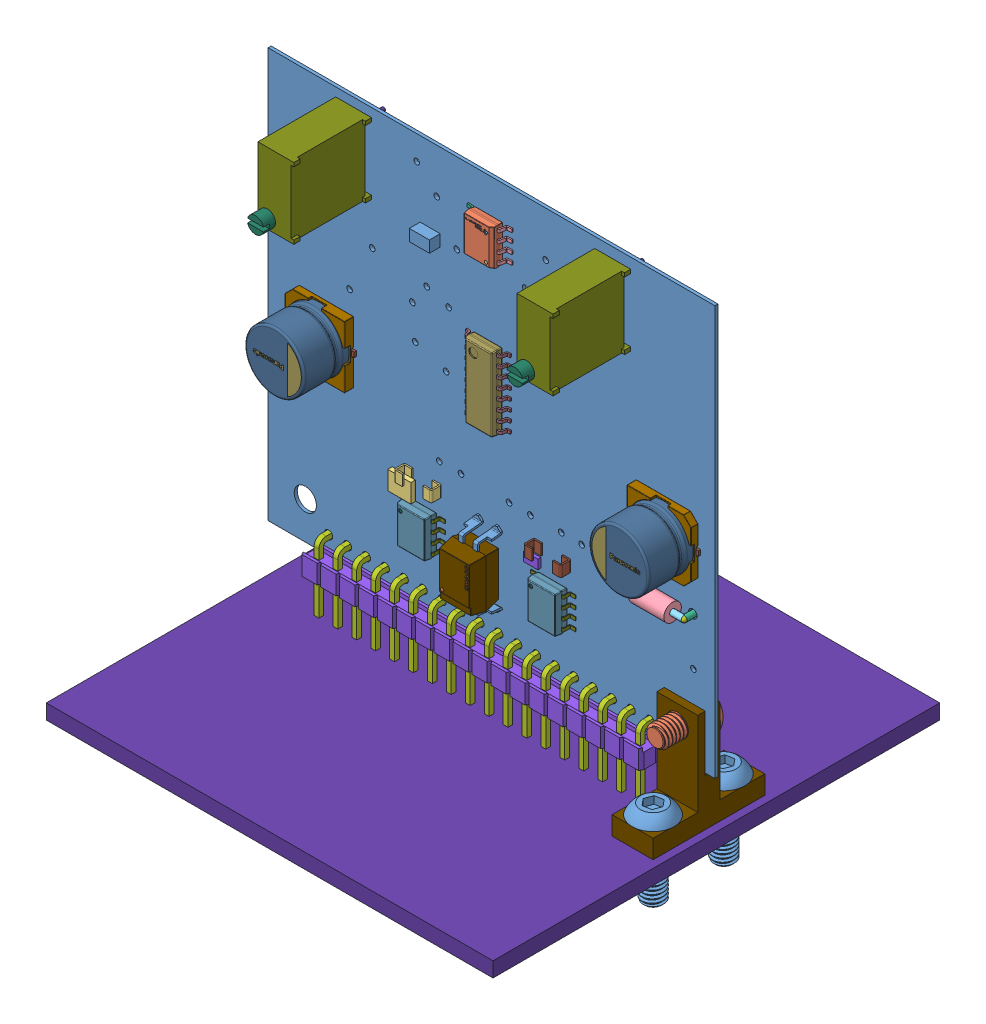
SolidWorks assembly Макет PWM, configuration Default. Lengths in mm.
Overall size (60 68.93 60).
439 component instances, 56 part files, 6 mates.
Components (placement in the parent):
- PWM_controller-1: PWM_controller [Default] at (-319.0135 -82.8288 51.7656) size (60 62.62 16.05)
  - PWM_controller.step-1: PWM_controller.step [Default] at origin size (60 62.62 16.05)
    - Board.step-1: Board.step [Default] at origin size (60 55 0.41)
      - Open CASCADE STEP translator 6.8 2.1.1.step-1: Open CASCADE STEP translator 6.8 2.1.1.step [Default] at (0 0 -0.4115) size (60 55 0.41)
    - R32.step-1: R32.step [Default] at origin size (3.2 2.5 0.7)
      - Res_Stackpole_Electronics_RMCF1210JT5K10_eec.step-1: Res_Stackpole_Electronics_RMCF1210JT5K10_eec.step [Default] at (249.8598 58.1914 -0.4115) x (-1 0 0) z (0 0 -1) size (3.2 2.5 0.7)
        - terminals.step-1: terminals.step [Default] at origin size (3.2 2.5 0.7)
        - body.step-1: body.step [Default] at origin size (3.1 2.5 0.6)
        - top.step-1: top.step [Default] at (-0.71 0 0.65) size (2.2 2.5 0.05)
        - logo.step-1: logo.step [Default] at (0 0 0.7) size (1.25 0.57 0)
    - C2.step-1: C2.step [Default] at origin size (2.7 3.4 1)
      - 6948496496.step-1: 6948496496.step [Default] at (219.9386 58.9514 -1.4115) size (2.7 0.5 1)
        - Extruded.step-1: Extruded.step [Default] at origin size (2.7 0.5 1)
      - 6948496496.step-2: 6948496496.step [Default] at (219.9386 61.8514 -1.4115) size (2.7 0.5 1)
        - Extruded.step-1: Extruded.step [Default] at origin size (2.7 0.5 1)
      - 6948486416.step-1: 6948486416.step [Default] at (219.9386 60.4014 -1.4115) size (2.7 2.4 1)
        - Extruded-0.step-1: Extruded-0.step [Default] at origin size (2.7 2.4 1)
    - C1.step-1: C1.step [Default] at origin size (2.7 3.4 1)
      - 6948496496.step-1: 6948496496.step [Default] at (237.0328 57.9862 -1.4115) size (2.7 0.5 1)
        - Extruded.step-1: Extruded.step [Default] at origin size (2.7 0.5 1)
      - 6948496496.step-2: 6948496496.step [Default] at (237.0328 60.8862 -1.4115) size (2.7 0.5 1)
        - Extruded.step-1: Extruded.step [Default] at origin size (2.7 0.5 1)
      - 6948486416.step-1: 6948486416.step [Default] at (237.0328 59.4362 -1.4115) size (2.7 2.4 1)
        - Extruded-0.step-1: Extruded-0.step [Default] at origin size (2.7 2.4 1)
    - R31.step-1: R31.step [Default] at origin size (1.25 2 0.5)
      - Res_Vishay_CRCW0805100KFKEA_eec.step-1: Res_Vishay_CRCW0805100KFKEA_eec.step [Default] at (205.232 89.4842 -0.4115) x (0 1 0) z (0 0 -1) size (2 1.25 0.5)
        - body-1.step-1: body-1.step [Default] at (0 0 0.45) x (1 0 0) z (0 0 -1) size (1.9 1.25 0.4)
        - pad.step-1: pad.step [Default] at (-0.8133 -0.625 0.5) x (1 0 0) z (0 1 0) size (0.3 0.5 1.25)
        - pad.step-2: pad.step [Default] at (0.8133 0.625 0.5) x (-1 0 0) z (0 -1 0) size (0.3 0.5 1.25)
        - top-2.step-1: top-2.step [Default] at (0 0 0.05) x (1 0 0) z (0 0 -1) size (1.4 1.25 0.05)
        - top-2.step-2: top-2.step [Default] at (0 0 0.5) x (1 0 0) z (0 0 -1) size (1.4 1.25 0.05)
        - Vishay.step-1: Vishay.step [Default] at (0.032 -0.7832 0.5) size (0.44 0.37 0)
    - R4.step-1: R4.step [Default] at origin size (1.25 2 0.5)
      - Res_Vishay_CRCW0805100KFKEA_eec.step-1: Res_Vishay_CRCW0805100KFKEA_eec.step [Default] at (206.9846 87.503 -0.4115) x (0 -1 0) z (0 0 -1) size (2 1.25 0.5)
        - body-1.step-1: body-1.step [Default] at (0 0 0.45) x (1 0 0) z (0 0 -1) size (1.9 1.25 0.4)
        - pad.step-1: pad.step [Default] at (-0.8133 -0.625 0.5) x (1 0 0) z (0 1 0) size (0.3 0.5 1.25)
        - pad.step-2: pad.step [Default] at (0.8133 0.625 0.5) x (-1 0 0) z (0 -1 0) size (0.3 0.5 1.25)
        - top-2.step-1: top-2.step [Default] at (0 0 0.05) x (1 0 0) z (0 0 -1) size (1.4 1.25 0.05)
        - top-2.step-2: top-2.step [Default] at (0 0 0.5) x (1 0 0) z (0 0 -1) size (1.4 1.25 0.05)
        - Vishay.step-1: Vishay.step [Default] at (0.032 -0.7832 0.5) size (0.44 0.37 0)
    - R3.step-1: R3.step [Default] at origin size (1.25 2 0.5)
      - Res_Vishay_CRCW0805100KFKEA_eec.step-1: Res_Vishay_CRCW0805100KFKEA_eec.step [Default] at (210.3628 76.8604 -0.4115) x (0 -1 0) z (0 0 -1) size (2 1.25 0.5)
        - body-1.step-1: body-1.step [Default] at (0 0 0.45) x (1 0 0) z (0 0 -1) size (1.9 1.25 0.4)
        - pad.step-1: pad.step [Default] at (-0.8133 -0.625 0.5) x (1 0 0) z (0 1 0) size (0.3 0.5 1.25)
        - pad.step-2: pad.step [Default] at (0.8133 0.625 0.5) x (-1 0 0) z (0 -1 0) size (0.3 0.5 1.25)
        - top-2.step-1: top-2.step [Default] at (0 0 0.05) x (1 0 0) z (0 0 -1) size (1.4 1.25 0.05)
        - top-2.step-2: top-2.step [Default] at (0 0 0.5) x (1 0 0) z (0 0 -1) size (1.4 1.25 0.05)
        - Vishay.step-1: Vishay.step [Default] at (0.032 -0.7832 0.5) size (0.44 0.37 0)
    - R2.step-1: R2.step [Default] at origin size (1.25 2 0.5)
      - Res_Vishay_CRCW0805100KFKEA_eec.step-1: Res_Vishay_CRCW0805100KFKEA_eec.step [Default] at (223.7232 76.7588 -0.4115) x (0 -1 0) z (0 0 -1) size (2 1.25 0.5)
        - body-1.step-1: body-1.step [Default] at (0 0 0.45) x (1 0 0) z (0 0 -1) size (1.9 1.25 0.4)
        - pad.step-1: pad.step [Default] at (-0.8133 -0.625 0.5) x (1 0 0) z (0 1 0) size (0.3 0.5 1.25)
        - pad.step-2: pad.step [Default] at (0.8133 0.625 0.5) x (-1 0 0) z (0 -1 0) size (0.3 0.5 1.25)
        - top-2.step-1: top-2.step [Default] at (0 0 0.05) x (1 0 0) z (0 0 -1) size (1.4 1.25 0.05)
        - top-2.step-2: top-2.step [Default] at (0 0 0.5) x (1 0 0) z (0 0 -1) size (1.4 1.25 0.05)
        - Vishay.step-1: Vishay.step [Default] at (0.032 -0.7832 0.5) size (0.44 0.37 0)
    - R1.step-1: R1.step [Default] at origin size (1.25 2 0.5)
      - Res_Vishay_CRCW0805100KFKEA_eec.step-1: Res_Vishay_CRCW0805100KFKEA_eec.step [Default] at (225.7044 76.7842 -0.4115) x (0 1 0) z (0 0 -1) size (2 1.25 0.5)
        - body-1.step-1: body-1.step [Default] at (0 0 0.45) x (1 0 0) z (0 0 -1) size (1.9 1.25 0.4)
        - pad.step-1: pad.step [Default] at (-0.8133 -0.625 0.5) x (1 0 0) z (0 1 0) size (0.3 0.5 1.25)
        - pad.step-2: pad.step [Default] at (0.8133 0.625 0.5) x (-1 0 0) z (0 -1 0) size (0.3 0.5 1.25)
        - top-2.step-1: top-2.step [Default] at (0 0 0.05) x (1 0 0) z (0 0 -1) size (1.4 1.25 0.05)
        - top-2.step-2: top-2.step [Default] at (0 0 0.5) x (1 0 0) z (0 0 -1) size (1.4 1.25 0.05)
        - Vishay.step-1: Vishay.step [Default] at (0.032 -0.7832 0.5) size (0.44 0.37 0)
    - R30.step-1: R30.step [Default] at origin size (1.25 2 0.5)
      - Res_Vishay_CRCW0805100KFKEA_eec.step-1: Res_Vishay_CRCW0805100KFKEA_eec.step [Default] at (220.9546 82.6008 -0.4115) x (0 -1 0) z (0 0 -1) size (2 1.25 0.5)
        - body-1.step-1: body-1.step [Default] at (0 0 0.45) x (1 0 0) z (0 0 -1) size (1.9 1.25 0.4)
        - pad.step-1: pad.step [Default] at (-0.8133 -0.625 0.5) x (1 0 0) z (0 1 0) size (0.3 0.5 1.25)
        - pad.step-2: pad.step [Default] at (0.8133 0.625 0.5) x (-1 0 0) z (0 -1 0) size (0.3 0.5 1.25)
        - top-2.step-1: top-2.step [Default] at (0 0 0.05) x (1 0 0) z (0 0 -1) size (1.4 1.25 0.05)
        - top-2.step-2: top-2.step [Default] at (0 0 0.5) x (1 0 0) z (0 0 -1) size (1.4 1.25 0.05)
        - Vishay.step-1: Vishay.step [Default] at (0.032 -0.7832 0.5) size (0.44 0.37 0)
    - R29.step-1: R29.step [Default] at origin size (1.25 2 0.5)
      - Res_Vishay_CRCW0805100KFKEA_eec.step-1: Res_Vishay_CRCW0805100KFKEA_eec.step [Default] at (211.2772 90.4084 -0.4115) x (0 -1 0) z (0 0 -1) size (2 1.25 0.5)
        - body-1.step-1: body-1.step [Default] at (0 0 0.45) x (1 0 0) z (0 0 -1) size (1.9 1.25 0.4)
        - pad.step-1: pad.step [Default] at (-0.8133 -0.625 0.5) x (1 0 0) z (0 1 0) size (0.3 0.5 1.25)
        - pad.step-2: pad.step [Default] at (0.8133 0.625 0.5) x (-1 0 0) z (0 -1 0) size (0.3 0.5 1.25)
        - top-2.step-1: top-2.step [Default] at (0 0 0.05) x (1 0 0) z (0 0 -1) size (1.4 1.25 0.05)
        - top-2.step-2: top-2.step [Default] at (0 0 0.5) x (1 0 0) z (0 0 -1) size (1.4 1.25 0.05)
        - Vishay.step-1: Vishay.step [Default] at (0.032 -0.7832 0.5) size (0.44 0.37 0)
    - R28.step-1: R28.step [Default] at origin size (2 1.25 0.5)
      - Res_Vishay_CRCW0805100KFKEA_eec.step-1: Res_Vishay_CRCW0805100KFKEA_eec.step [Default] at (224.0026 85.6742 -0.4115) x (-1 0 0) z (0 0 -1) size (2 1.25 0.5)
        - body-1.step-1: body-1.step [Default] at (0 0 0.45) x (1 0 0) z (0 0 -1) size (1.9 1.25 0.4)
        - pad.step-1: pad.step [Default] at (-0.8133 -0.625 0.5) x (1 0 0) z (0 1 0) size (0.3 0.5 1.25)
        - pad.step-2: pad.step [Default] at (0.8133 0.625 0.5) x (-1 0 0) z (0 -1 0) size (0.3 0.5 1.25)
        - top-2.step-1: top-2.step [Default] at (0 0 0.05) x (1 0 0) z (0 0 -1) size (1.4 1.25 0.05)
        - top-2.step-2: top-2.step [Default] at (0 0 0.5) x (1 0 0) z (0 0 -1) size (1.4 1.25 0.05)
        - Vishay.step-1: Vishay.step [Default] at (0.032 -0.7832 0.5) size (0.44 0.37 0)
    - R27.step-1: R27.step [Default] at origin size (1.25 2 0.5)
      - Res_Vishay_CRCW0805100KFKEA_eec.step-1: Res_Vishay_CRCW0805100KFKEA_eec.step [Default] at (213.7156 87.5792 -0.4115) x (0 -1 0) z (0 0 -1) size (2 1.25 0.5)
        - body-1.step-1: body-1.step [Default] at (0 0 0.45) x (1 0 0) z (0 0 -1) size (1.9 1.25 0.4)
        - pad.step-1: pad.step [Default] at (-0.8133 -0.625 0.5) x (1 0 0) z (0 1 0) size (0.3 0.5 1.25)
        - pad.step-2: pad.step [Default] at (0.8133 0.625 0.5) x (-1 0 0) z (0 -1 0) size (0.3 0.5 1.25)
        - top-2.step-1: top-2.step [Default] at (0 0 0.05) x (1 0 0) z (0 0 -1) size (1.4 1.25 0.05)
        - top-2.step-2: top-2.step [Default] at (0 0 0.5) x (1 0 0) z (0 0 -1) size (1.4 1.25 0.05)
        - Vishay.step-1: Vishay.step [Default] at (0.032 -0.7832 0.5) size (0.44 0.37 0)
    - C14.step-1: C14.step [Default] at origin size (1.25 2 0.88)
      - Cap_KEMET_C0805C472J3HAC_eec.step-1: Cap_KEMET_C0805C472J3HAC_eec.step [Default] at (211.2264 84.3788 -0.4115) x (0 1 0) z (0 0 -1) size (1 1.15 0.78)
      - Cap_KEMET_C0805C472J3HAC_eec-3.step-1: Cap_KEMET_C0805C472J3HAC_eec-3.step [Default] at (211.2264 84.3788 -0.4115) x (0 1 0) z (0 0 -1) size (2 1.25 0.88)
      - Cap_KEMET_C0805C472J3HAC_eec-4.step-1: Cap_KEMET_C0805C472J3HAC_eec-4.step [Default] at (211.2264 84.3788 -0.4115) x (0 1 0) z (0 0 -1) size (0.59 0.12 0)
    - C13.step-1: C13.step [Default] at origin size (1.25 2 0.88)
      - Cap_KEMET_C0805C472J3HAC_eec.step-1: Cap_KEMET_C0805C472J3HAC_eec.step [Default] at (213.6648 84.3788 -0.4115) x (0 -1 0) z (0 0 -1) size (1 1.15 0.78)
      - Cap_KEMET_C0805C472J3HAC_eec-3.step-1: Cap_KEMET_C0805C472J3HAC_eec-3.step [Default] at (213.6648 84.3788 -0.4115) x (0 -1 0) z (0 0 -1) size (2 1.25 0.88)
      - Cap_KEMET_C0805C472J3HAC_eec-4.step-1: Cap_KEMET_C0805C472J3HAC_eec-4.step [Default] at (213.6648 84.3788 -0.4115) x (0 -1 0) z (0 0 -1) size (0.59 0.12 0)
    - R21.step-1: R21.step [Default] at origin size (2 1.25 0.5)
      - Res_Vishay_CRCW0805100KFKEA_eec.step-1: Res_Vishay_CRCW0805100KFKEA_eec.step [Default] at (225.0694 92.8624 -0.4115) x (1 0 0) z (0 0 -1) size (2 1.25 0.5)
        - body-1.step-1: body-1.step [Default] at (0 0 0.45) x (1 0 0) z (0 0 -1) size (1.9 1.25 0.4)
        - pad.step-1: pad.step [Default] at (-0.8133 -0.625 0.5) x (1 0 0) z (0 1 0) size (0.3 0.5 1.25)
        - pad.step-2: pad.step [Default] at (0.8133 0.625 0.5) x (-1 0 0) z (0 -1 0) size (0.3 0.5 1.25)
        - top-2.step-1: top-2.step [Default] at (0 0 0.05) x (1 0 0) z (0 0 -1) size (1.4 1.25 0.05)
        - top-2.step-2: top-2.step [Default] at (0 0 0.5) x (1 0 0) z (0 0 -1) size (1.4 1.25 0.05)
        - Vishay.step-1: Vishay.step [Default] at (0.032 -0.7832 0.5) size (0.44 0.37 0)
    - R20.step-1: R20.step [Default] at origin size (1.25 2 0.5)
      - Res_Vishay_CRCW0805100KFKEA_eec.step-1: Res_Vishay_CRCW0805100KFKEA_eec.step [Default] at (216.7382 97.3074 -0.4115) x (0 -1 0) z (0 0 -1) size (2 1.25 0.5)
        - body-1.step-1: body-1.step [Default] at (0 0 0.45) x (1 0 0) z (0 0 -1) size (1.9 1.25 0.4)
        - pad.step-1: pad.step [Default] at (-0.8133 -0.625 0.5) x (1 0 0) z (0 1 0) size (0.3 0.5 1.25)
        - pad.step-2: pad.step [Default] at (0.8133 0.625 0.5) x (-1 0 0) z (0 -1 0) size (0.3 0.5 1.25)
        - top-2.step-1: top-2.step [Default] at (0 0 0.05) x (1 0 0) z (0 0 -1) size (1.4 1.25 0.05)
        - top-2.step-2: top-2.step [Default] at (0 0 0.5) x (1 0 0) z (0 0 -1) size (1.4 1.25 0.05)
        - Vishay.step-1: Vishay.step [Default] at (0.032 -0.7832 0.5) size (0.44 0.37 0)
    - R19.step-1: R19.step [Default] at origin size (4.83 9.53 16.05)
      - Res_Bourns_3296W-1-504LF_eec.step-1: Res_Bourns_3296W-1-504LF_eec.step [Default] at (210.3653 92.9274 10.0159) x (0 0 -1) z (-1 0 0) size (1.59 2.18 2.18)
      - Res_Bourns_3296W-1-504LF_eec-5.step-1: Res_Bourns_3296W-1-504LF_eec-5.step [Default] at (210.3653 92.9274 10.0159) x (0 0 -1) z (-1 0 0) size (10.46 9.53 4.83)
      - Res_Bourns_3296W-1-504LF_eec-6.step-1: Res_Bourns_3296W-1-504LF_eec-6.step [Default] at (210.3653 92.9274 10.0159) x (0 0 -1) z (-1 0 0) size (4.53 5.59 0.51)
      - Res_Bourns_3296W-1-504LF_eec-7.step-1: Res_Bourns_3296W-1-504LF_eec-7.step [Default] at (210.3653 92.9274 10.0159) x (0 0 -1) z (-1 0 0) size (0.78 6.02 0.01)
    - R18.step-1: R18.step [Default] at origin size (1.25 2 0.5)
      - Res_Vishay_CRCW0805100KFKEA_eec.step-1: Res_Vishay_CRCW0805100KFKEA_eec.step [Default] at (214.884 97.3328 -0.4115) x (0 -1 0) z (0 0 -1) size (2 1.25 0.5)
        - body-1.step-1: body-1.step [Default] at (0 0 0.45) x (1 0 0) z (0 0 -1) size (1.9 1.25 0.4)
        - pad.step-1: pad.step [Default] at (-0.8133 -0.625 0.5) x (1 0 0) z (0 1 0) size (0.3 0.5 1.25)
        - pad.step-2: pad.step [Default] at (0.8133 0.625 0.5) x (-1 0 0) z (0 -1 0) size (0.3 0.5 1.25)
        - top-2.step-1: top-2.step [Default] at (0 0 0.05) x (1 0 0) z (0 0 -1) size (1.4 1.25 0.05)
        - top-2.step-2: top-2.step [Default] at (0 0 0.5) x (1 0 0) z (0 0 -1) size (1.4 1.25 0.05)
        - Vishay.step-1: Vishay.step [Default] at (0.032 -0.7832 0.5) size (0.44 0.37 0)
    - R17.step-1: R17.step [Default] at origin size (2 1.25 0.5)
      - Res_Vishay_CRCW0805100KFKEA_eec.step-1: Res_Vishay_CRCW0805100KFKEA_eec.step [Default] at (222.631 97.6376 -0.4115) x (-1 0 0) z (0 0 -1) size (2 1.25 0.5)
        - body-1.step-1: body-1.step [Default] at (0 0 0.45) x (1 0 0) z (0 0 -1) size (1.9 1.25 0.4)
        - pad.step-1: pad.step [Default] at (-0.8133 -0.625 0.5) x (1 0 0) z (0 1 0) size (0.3 0.5 1.25)
        - pad.step-2: pad.step [Default] at (0.8133 0.625 0.5) x (-1 0 0) z (0 -1 0) size (0.3 0.5 1.25)
        - top-2.step-1: top-2.step [Default] at (0 0 0.05) x (1 0 0) z (0 0 -1) size (1.4 1.25 0.05)
        - top-2.step-2: top-2.step [Default] at (0 0 0.5) x (1 0 0) z (0 0 -1) size (1.4 1.25 0.05)
        - Vishay.step-1: Vishay.step [Default] at (0.032 -0.7832 0.5) size (0.44 0.37 0)
    - D5.step-1: D5.step [Default] at origin size (2.7 1.55 1.45)
      - 6038362448.step-1: 6038362448.step [Default] at (235.0262 92.964 0) size (2.7 1.55 1.45)
        - Extruded-8.step-1: Extruded-8.step [Default] at origin size (2.7 1.55 1.45)
    - D4.step-1: D4.step [Default] at origin size (2.7 1.55 1.45)
      - 6038362448.step-1: 6038362448.step [Default] at (218.6178 92.7862 0) size (2.7 1.55 1.45)
        - Extruded-8.step-1: Extruded-8.step [Default] at origin size (2.7 1.55 1.45)
    - C12.step-1: C12.step [Default] at origin size (2 1.25 0.88)
      - Cap_KEMET_C0805C472J3HAC_eec.step-1: Cap_KEMET_C0805C472J3HAC_eec.step [Default] at (237.2614 97.9424 -0.4115) x (1 0 0) z (0 0 -1) size (1 1.15 0.78)
      - Cap_KEMET_C0805C472J3HAC_eec-3.step-1: Cap_KEMET_C0805C472J3HAC_eec-3.step [Default] at (237.2614 97.9424 -0.4115) x (1 0 0) z (0 0 -1) size (2 1.25 0.88)
      - Cap_KEMET_C0805C472J3HAC_eec-4.step-1: Cap_KEMET_C0805C472J3HAC_eec-4.step [Default] at (237.2614 97.9424 -0.4115) x (1 0 0) z (0 0 -1) size (0.59 0.12 0)
    - C11.step-1: C11.step [Default] at origin size (1.25 2 0.88)
      - Cap_KEMET_C0805C472J3HAC_eec.step-1: Cap_KEMET_C0805C472J3HAC_eec.step [Default] at (212.6996 97.3836 -0.4115) x (0 -1 0) z (0 0 -1) size (1 1.15 0.78)
      - Cap_KEMET_C0805C472J3HAC_eec-3.step-1: Cap_KEMET_C0805C472J3HAC_eec-3.step [Default] at (212.6996 97.3836 -0.4115) x (0 -1 0) z (0 0 -1) size (2 1.25 0.88)
      - Cap_KEMET_C0805C472J3HAC_eec-4.step-1: Cap_KEMET_C0805C472J3HAC_eec-4.step [Default] at (212.6996 97.3836 -0.4115) x (0 -1 0) z (0 0 -1) size (0.59 0.12 0)
    - R25.step-1: R25.step [Default] at origin size (2 1.25 0.5)
      - Res_Vishay_CRCW0805100KFKEA_eec.step-1: Res_Vishay_CRCW0805100KFKEA_eec.step [Default] at (231.2416 97.663 -0.4115) x (-1 0 0) z (0 0 -1) size (2 1.25 0.5)
        - body-1.step-1: body-1.step [Default] at (0 0 0.45) x (1 0 0) z (0 0 -1) size (1.9 1.25 0.4)
        - pad.step-1: pad.step [Default] at (-0.8133 -0.625 0.5) x (1 0 0) z (0 1 0) size (0.3 0.5 1.25)
        - pad.step-2: pad.step [Default] at (0.8133 0.625 0.5) x (-1 0 0) z (0 -1 0) size (0.3 0.5 1.25)
        - top-2.step-1: top-2.step [Default] at (0 0 0.05) x (1 0 0) z (0 0 -1) size (1.4 1.25 0.05)
        - top-2.step-2: top-2.step [Default] at (0 0 0.5) x (1 0 0) z (0 0 -1) size (1.4 1.25 0.05)
        - Vishay.step-1: Vishay.step [Default] at (0.032 -0.7832 0.5) size (0.44 0.37 0)
    - R23.step-1: R23.step [Default] at origin size (2 1.25 0.5)
      - Res_Vishay_CRCW0805100KFKEA_eec.step-1: Res_Vishay_CRCW0805100KFKEA_eec.step [Default] at (237.2614 100.1268 -0.4115) x (1 0 0) z (0 0 -1) size (2 1.25 0.5)
        - body-1.step-1: body-1.step [Default] at (0 0 0.45) x (1 0 0) z (0 0 -1) size (1.9 1.25 0.4)
        - pad.step-1: pad.step [Default] at (-0.8133 -0.625 0.5) x (1 0 0) z (0 1 0) size (0.3 0.5 1.25)
        - pad.step-2: pad.step [Default] at (0.8133 0.625 0.5) x (-1 0 0) z (0 -1 0) size (0.3 0.5 1.25)
        - top-2.step-1: top-2.step [Default] at (0 0 0.05) x (1 0 0) z (0 0 -1) size (1.4 1.25 0.05)
        - top-2.step-2: top-2.step [Default] at (0 0 0.5) x (1 0 0) z (0 0 -1) size (1.4 1.25 0.05)
        - Vishay.step-1: Vishay.step [Default] at (0.032 -0.7832 0.5) size (0.44 0.37 0)
    - R26.step-1: R26.step [Default] at origin size (2 1.25 0.5)
      - Res_Vishay_CRCW0805100KFKEA_eec.step-1: Res_Vishay_CRCW0805100KFKEA_eec.step [Default] at (228.6508 92.8624 -0.4115) x (-1 0 0) z (0 0 -1) size (2 1.25 0.5)
        - body-1.step-1: body-1.step [Default] at (0 0 0.45) x (1 0 0) z (0 0 -1) size (1.9 1.25 0.4)
        - pad.step-1: pad.step [Default] at (-0.8133 -0.625 0.5) x (1 0 0) z (0 1 0) size (0.3 0.5 1.25)
        - pad.step-2: pad.step [Default] at (0.8133 0.625 0.5) x (-1 0 0) z (0 -1 0) size (0.3 0.5 1.25)
        - top-2.step-1: top-2.step [Default] at (0 0 0.05) x (1 0 0) z (0 0 -1) size (1.4 1.25 0.05)
        - top-2.step-2: top-2.step [Default] at (0 0 0.5) x (1 0 0) z (0 0 -1) size (1.4 1.25 0.05)
        - Vishay.step-1: Vishay.step [Default] at (0.032 -0.7832 0.5) size (0.44 0.37 0)
    - R22.step-1: R22.step [Default] at origin size (2 1.25 0.5)
      - Res_Vishay_CRCW0805100KFKEA_eec.step-1: Res_Vishay_CRCW0805100KFKEA_eec.step [Default] at (234.2388 95.2754 -0.4115) x (1 0 0) z (0 0 -1) size (2 1.25 0.5)
        - body-1.step-1: body-1.step [Default] at (0 0 0.45) x (1 0 0) z (0 0 -1) size (1.9 1.25 0.4)
        - pad.step-1: pad.step [Default] at (-0.8133 -0.625 0.5) x (1 0 0) z (0 1 0) size (0.3 0.5 1.25)
        - pad.step-2: pad.step [Default] at (0.8133 0.625 0.5) x (-1 0 0) z (0 -1 0) size (0.3 0.5 1.25)
        - top-2.step-1: top-2.step [Default] at (0 0 0.05) x (1 0 0) z (0 0 -1) size (1.4 1.25 0.05)
        - top-2.step-2: top-2.step [Default] at (0 0 0.5) x (1 0 0) z (0 0 -1) size (1.4 1.25 0.05)
        - Vishay.step-1: Vishay.step [Default] at (0.032 -0.7832 0.5) size (0.44 0.37 0)
    - R24.step-1: R24.step [Default] at origin size (4.83 9.53 16.05)
      - Res_Bourns_3296W-1-504LF_eec.step-1: Res_Bourns_3296W-1-504LF_eec.step [Default] at (245.1683 92.6988 10.0159) x (0 0 -1) z (-1 0 0) size (1.59 2.18 2.18)
      - Res_Bourns_3296W-1-504LF_eec-5.step-1: Res_Bourns_3296W-1-504LF_eec-5.step [Default] at (245.1683 92.6988 10.0159) x (0 0 -1) z (-1 0 0) size (10.46 9.53 4.83)
      - Res_Bourns_3296W-1-504LF_eec-6.step-1: Res_Bourns_3296W-1-504LF_eec-6.step [Default] at (245.1683 92.6988 10.0159) x (0 0 -1) z (-1 0 0) size (4.53 5.59 0.51)
      - Res_Bourns_3296W-1-504LF_eec-7.step-1: Res_Bourns_3296W-1-504LF_eec-7.step [Default] at (245.1683 92.6988 10.0159) x (0 0 -1) z (-1 0 0) size (0.78 6.02 0.01)
    - U4.step-1: U4.step [Default] at origin size (6 4.9 1.76)
      - IC_Texas_Instruments_ISO7220ADR_eec.step-1: IC_Texas_Instruments_ISO7220ADR_eec.step [Default] at (226.7712 96.9772 0) x (-1 0 0) z (0 0 1) size (6 4.9 1.76)
        - IC_BODY.step-1: IC_BODY.step [Default] at (0 0 0.25) x (0 -1 0) z (0 0 1) size (4.9 3.9 1.5)
        - circle.step-1: circle.step [Default] at (-1.0726 1.9393 1.751) x (1 0 0) z (0 0 -1) size (0.4 0.4 0)
        - IC_LEG.step-1: IC_LEG.step [Default] at (-3 2.1095 0) x (1 0 0) z (0 -1 0) size (1.15 1.11 0.41)
        - IC_LEG.step-2: IC_LEG.step [Default] at (-3 0.8395 0) x (1 0 0) z (0 -1 0) size (1.15 1.11 0.41)
        - IC_LEG.step-3: IC_LEG.step [Default] at (-3 -0.4305 0) x (1 0 0) z (0 -1 0) size (1.15 1.11 0.41)
        - IC_LEG.step-4: IC_LEG.step [Default] at (-3 -1.7005 0) x (1 0 0) z (0 -1 0) size (1.15 1.11 0.41)
        - Texas_Instruments.step-1: Texas_Instruments.step [Default] at (0.0232 -1.7093 1.75) size (3.04 0.71 0.02)
        - IC_LEG_MIR8.step-1: IC_LEG_MIR8.step [Default] at (3 2.1095 0) x (-1 0 0) z (0 1 0) size (1.15 1.11 0.41)
        - IC_LEG_MIR8.step-2: IC_LEG_MIR8.step [Default] at (3 0.8395 0) x (-1 0 0) z (0 1 0) size (1.15 1.11 0.41)
        - IC_LEG_MIR8.step-3: IC_LEG_MIR8.step [Default] at (3 -0.4305 0) x (-1 0 0) z (0 1 0) size (1.15 1.11 0.41)
        - IC_LEG_MIR8.step-4: IC_LEG_MIR8.step [Default] at (3 -1.7005 0) x (-1 0 0) z (0 1 0) size (1.15 1.11 0.41)
    - P2.step-1: P2.step [Default] at origin size (45.72 10.36 5.54)
      - 61301811021.step-1: 61301811021.step [Default] at (226.5681 48.2841 1.31) x (-1 0 0) z (0 -1 0) size (45.72 5.54 10.36)
        - 6130xx11021_PIN.step-1: 6130xx11021_PIN.step [Default] at (-21.59 0 2.09) size (0.64 4.59 10.36)
        - 6130xx11021_PIN.step-2: 6130xx11021_PIN.step [Default] at (-19.05 0 2.09) size (0.64 4.59 10.36)
        - 6130xx11021_PIN.step-3: 6130xx11021_PIN.step [Default] at (-16.51 0 2.09) size (0.64 4.59 10.36)
        - 6130xx11021_PIN.step-4: 6130xx11021_PIN.step [Default] at (-13.97 0 2.09) size (0.64 4.59 10.36)
        - 6130xx11021_PIN.step-5: 6130xx11021_PIN.step [Default] at (-11.43 0 2.09) size (0.64 4.59 10.36)
        - 6130xx11021_PIN.step-6: 6130xx11021_PIN.step [Default] at (-8.89 0 2.09) size (0.64 4.59 10.36)
        - 6130xx11021_PIN.step-7: 6130xx11021_PIN.step [Default] at (-6.35 0 2.09) size (0.64 4.59 10.36)
        - 6130xx11021_PIN.step-8: 6130xx11021_PIN.step [Default] at (-3.81 0 2.09) size (0.64 4.59 10.36)
        - 6130xx11021_PIN.step-9: 6130xx11021_PIN.step [Default] at (-1.27 0 2.09) size (0.64 4.59 10.36)
        - 6130xx11021_PIN.step-10: 6130xx11021_PIN.step [Default] at (1.27 0 2.09) size (0.64 4.59 10.36)
        - 6130xx11021_PIN.step-11: 6130xx11021_PIN.step [Default] at (3.81 0 2.09) size (0.64 4.59 10.36)
        - 6130xx11021_PIN.step-12: 6130xx11021_PIN.step [Default] at (6.35 0 2.09) size (0.64 4.59 10.36)
        - 6130xx11021_PIN.step-13: 6130xx11021_PIN.step [Default] at (8.89 0 2.09) size (0.64 4.59 10.36)
        - 6130xx11021_PIN.step-14: 6130xx11021_PIN.step [Default] at (11.43 0 2.09) size (0.64 4.59 10.36)
        - 6130xx11021_PIN.step-15: 6130xx11021_PIN.step [Default] at (13.97 0 2.09) size (0.64 4.59 10.36)
        - 6130xx11021_PIN.step-16: 6130xx11021_PIN.step [Default] at (16.51 0 2.09) size (0.64 4.59 10.36)
        - 6130xx11021_PIN.step-17: 6130xx11021_PIN.step [Default] at (19.05 0 2.09) size (0.64 4.59 10.36)
        - 6130xx11021_PIN.step-18: 6130xx11021_PIN.step [Default] at (21.59 0 2.09) size (0.64 4.59 10.36)
        - 61301811021-9.step-1: 61301811021-9.step [Default] at origin size (45.72 2.54 2.54)
    - R5.step-1: R5.step [Default] at origin size (1.25 2 0.5)
      - Res_Vishay_CRCW0805100KFKEA_eec.step-1: Res_Vishay_CRCW0805100KFKEA_eec.step [Default] at (208.788 84.3378 -0.4115) x (0 -1 0) z (0 0 -1) size (2 1.25 0.5)
        - body-1.step-1: body-1.step [Default] at (0 0 0.45) x (1 0 0) z (0 0 -1) size (1.9 1.25 0.4)
        - pad.step-1: pad.step [Default] at (-0.8133 -0.625 0.5) x (1 0 0) z (0 1 0) size (0.3 0.5 1.25)
        - pad.step-2: pad.step [Default] at (0.8133 0.625 0.5) x (-1 0 0) z (0 -1 0) size (0.3 0.5 1.25)
        - top-2.step-1: top-2.step [Default] at (0 0 0.05) x (1 0 0) z (0 0 -1) size (1.4 1.25 0.05)
        - top-2.step-2: top-2.step [Default] at (0 0 0.5) x (1 0 0) z (0 0 -1) size (1.4 1.25 0.05)
        - Vishay.step-1: Vishay.step [Default] at (0.032 -0.7832 0.5) size (0.44 0.37 0)
    - R9.step-1: R9.step [Default] at origin size (1.25 2 0.5)
      - Res_Vishay_CRCW0805100KFKEA_eec.step-1: Res_Vishay_CRCW0805100KFKEA_eec.step [Default] at (206.9592 84.328 -0.4115) x (0 1 0) z (0 0 -1) size (2 1.25 0.5)
        - body-1.step-1: body-1.step [Default] at (0 0 0.45) x (1 0 0) z (0 0 -1) size (1.9 1.25 0.4)
        - pad.step-1: pad.step [Default] at (-0.8133 -0.625 0.5) x (1 0 0) z (0 1 0) size (0.3 0.5 1.25)
        - pad.step-2: pad.step [Default] at (0.8133 0.625 0.5) x (-1 0 0) z (0 -1 0) size (0.3 0.5 1.25)
        - top-2.step-1: top-2.step [Default] at (0 0 0.05) x (1 0 0) z (0 0 -1) size (1.4 1.25 0.05)
        - top-2.step-2: top-2.step [Default] at (0 0 0.5) x (1 0 0) z (0 0 -1) size (1.4 1.25 0.05)
        - Vishay.step-1: Vishay.step [Default] at (0.032 -0.7832 0.5) size (0.44 0.37 0)
    - R6.step-1: R6.step [Default] at origin size (3.2 2.5 0.7)
      - Res_Stackpole_Electronics_RMCF1210JT5K10_eec.step-1: Res_Stackpole_Electronics_RMCF1210JT5K10_eec.step [Default] at (249.8854 61.6712 -0.4115) x (-1 0 0) z (0 0 -1) size (3.2 2.5 0.7)
        - terminals.step-1: terminals.step [Default] at origin size (3.2 2.5 0.7)
        - body.step-1: body.step [Default] at origin size (3.1 2.5 0.6)
        - top.step-1: top.step [Default] at (-0.71 0 0.65) size (2.2 2.5 0.05)
        - logo.step-1: logo.step [Default] at (0 0 0.7) size (1.25 0.57 0)
    - C5.step-1: C5.step [Default] at origin size (9 8.3 6.5)
      - Cap_Panasonic_Electronic_Components_EEE-FK1H101GP_eec.step-1: Cap_Panasonic_Electronic_Components_EEE-FK1H101GP_eec.step [Default] at (204.216 73.9902 0) x (-1 0 0) z (0 0 1) size (9 8.3 6.5)
        - base.step-1: base.step [Default] at origin size (8.3 8.3 1.25)
        - cap.step-1: cap.step [Default] at origin size (8 8 6)
        - pins.step-1: pins.step [Default] at origin size (9 0.65 0.3)
        - logo-10.step-1: logo-10.step [Default] at (0 0 6.5) size (6.48 6.34 0)
    - C6.step-1: C6.step [Default] at origin size (2.7 3.4 1)
      - 6948496496.step-1: 6948496496.step [Default] at (213.487 78.9708 -1.4115) size (2.7 0.5 1)
        - Extruded.step-1: Extruded.step [Default] at origin size (2.7 0.5 1)
      - 6948496496.step-2: 6948496496.step [Default] at (213.487 76.0708 -1.4115) size (2.7 0.5 1)
        - Extruded.step-1: Extruded.step [Default] at origin size (2.7 0.5 1)
      - 6948486416.step-1: 6948486416.step [Default] at (213.487 77.5208 -1.4115) size (2.7 2.4 1)
        - Extruded-0.step-1: Extruded-0.step [Default] at origin size (2.7 2.4 1)
    - C7.step-1: C7.step [Default] at origin size (1.25 2 0.88)
      - Cap_KEMET_C0805C472J3HAC_eec.step-1: Cap_KEMET_C0805C472J3HAC_eec.step [Default] at (216.662 76.6318 -0.4115) x (0 -1 0) z (0 0 -1) size (1 1.15 0.78)
